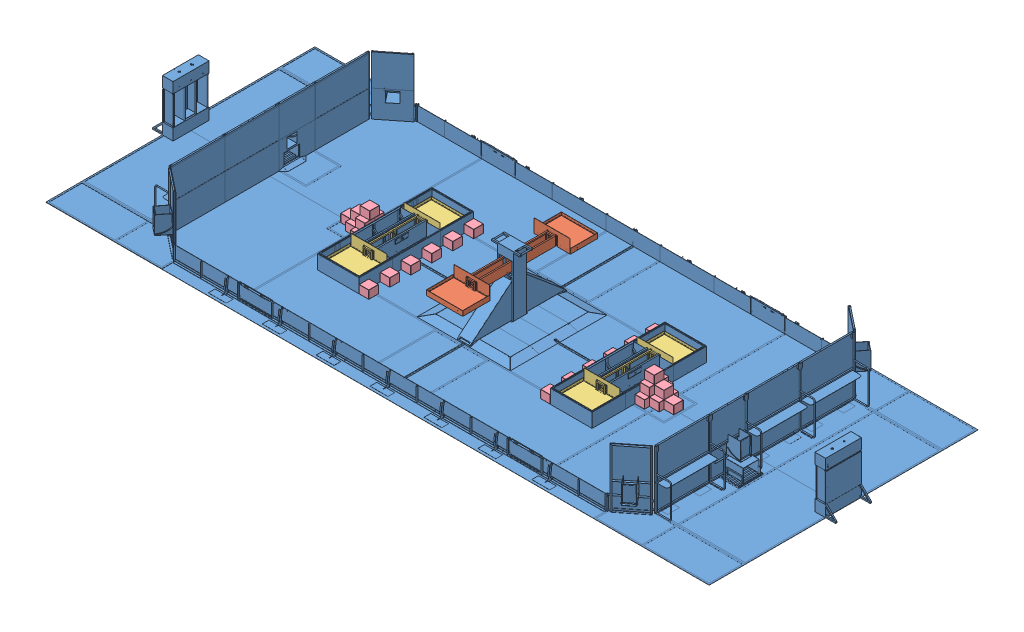
SolidWorks assembly FRC Field 2018a, configuration Arms Level. Lengths in mm.
Overall size (23234.65 2142.03 9144.04).
36 component instances, 4 part files, 15 mates.
Components (placement in the parent):
- FRC Fixed Field 2018-1: FRC Fixed Field 2018 [Default] at origin size (23234.65 2142.03 9144.04)
- Scale Arm-2: Scale Arm [Default] at (0 -0.1252 2.4571) x (1 0 0) z (0 0.001347 0.999999) size (1245.02 510 4602.7)
- Switch Arm-1: Switch Arm [Default] at (3962.4 0 -0.2032) size (1245.02 508 3684.03)
- Switch Arm-2: Switch Arm [Default] at (-3962.4 0 0) size (1245.02 508 3684.03)
- PowerUp Cube-1: PowerUp Cube [Default] at (4673.6 0 495.3) size (330.2 279.4 330.2)
- PowerUp Cube-2: PowerUp Cube [Default] at (4673.6 0 165.1) size (330.2 279.4 330.2)
- PowerUp Cube-3: PowerUp Cube [Default] at (4673.6 0 -165.1) size (330.2 279.4 330.2)
- PowerUp Cube-4: PowerUp Cube [Default] at (5003.8 0 330.2) size (330.2 279.4 330.2)
- PowerUp Cube-5: PowerUp Cube [Default] at (5003.8 0 0) size (330.2 279.4 330.2)
- PowerUp Cube-6: PowerUp Cube [Default] at (5334 0 165.1) size (330.2 279.4 330.2)
- PowerUp Cube-7: PowerUp Cube [Default] at (4673.6 279.4 330.2) size (330.2 279.4 330.2)
- PowerUp Cube-8: PowerUp Cube [Default] at (4673.6 279.4 0) size (330.2 279.4 330.2)
- PowerUp Cube-9: PowerUp Cube [Default] at (5003.8 279.4 165.1) size (330.2 279.4 330.2)
- PowerUp Cube-10: PowerUp Cube [Default] at (4673.6 558.8 165.1) size (330.2 279.4 330.2)
- PowerUp Cube-11: PowerUp Cube [Default] at (2921 0 -1619.25) size (330.2 279.4 330.2)
- PowerUp Cube-12: PowerUp Cube [Default] at (2921 0 -905.51) size (330.2 279.4 330.2)
- PowerUp Cube-13: PowerUp Cube [Default] at (2921 0 -191.77) size (330.2 279.4 330.2)
- PowerUp Cube-14: PowerUp Cube [Default] at (2921 0 521.97) size (330.2 279.4 330.2)
- PowerUp Cube-15: PowerUp Cube [Default] at (2921 0 1235.71) size (330.2 279.4 330.2)
- PowerUp Cube-16: PowerUp Cube [Default] at (2921 0 1949.45) size (330.2 279.4 330.2)
- PowerUp Cube-17: PowerUp Cube [Default] at (-4673.6 0 165.1) x (-1 0 0) z (0 0 -1) size (330.2 279.4 330.2)
- PowerUp Cube-18: PowerUp Cube [Default] at (-4673.6 0 -165.1) x (-1 0 0) z (0 0 -1) size (330.2 279.4 330.2)
- PowerUp Cube-19: PowerUp Cube [Default] at (-4673.6 0 -495.3) x (-1 0 0) z (0 0 -1) size (330.2 279.4 330.2)
- PowerUp Cube-20: PowerUp Cube [Default] at (-5003.8 0 0) x (-1 0 0) z (0 0 -1) size (330.2 279.4 330.2)
- PowerUp Cube-21: PowerUp Cube [Default] at (-5003.8 0 -330.2) x (-1 0 0) z (0 0 -1) size (330.2 279.4 330.2)
- PowerUp Cube-22: PowerUp Cube [Default] at (-5334 0 -165.1) x (-1 0 0) z (0 0 -1) size (330.2 279.4 330.2)
- PowerUp Cube-23: PowerUp Cube [Default] at (-4673.6 279.4 0) x (-1 0 0) z (0 0 -1) size (330.2 279.4 330.2)
- PowerUp Cube-24: PowerUp Cube [Default] at (-4673.6 279.4 -330.2) x (-1 0 0) z (0 0 -1) size (330.2 279.4 330.2)
- PowerUp Cube-25: PowerUp Cube [Default] at (-5003.8 279.4 -165.1) x (-1 0 0) z (0 0 -1) size (330.2 279.4 330.2)
- PowerUp Cube-26: PowerUp Cube [Default] at (-4673.6 558.8 -165.1) x (-1 0 0) z (0 0 -1) size (330.2 279.4 330.2)
- PowerUp Cube-27: PowerUp Cube [Default] at (-2921 0 -1949.45) x (-1 0 0) z (0 0 -1) size (330.2 279.4 330.2)
- PowerUp Cube-28: PowerUp Cube [Default] at (-2921 0 -1235.71) x (-1 0 0) z (0 0 -1) size (330.2 279.4 330.2)
- PowerUp Cube-29: PowerUp Cube [Default] at (-2921 0 -521.97) x (-1 0 0) z (0 0 -1) size (330.2 279.4 330.2)
- PowerUp Cube-30: PowerUp Cube [Default] at (-2921 0 191.77) x (-1 0 0) z (0 0 -1) size (330.2 279.4 330.2)
- PowerUp Cube-31: PowerUp Cube [Default] at (-2921 0 905.51) x (-1 0 0) z (0 0 -1) size (330.2 279.4 330.2)
- PowerUp Cube-32: PowerUp Cube [Default] at (-2921 0 1619.25) x (-1 0 0) z (0 0 -1) size (330.2 279.4 330.2)
Mates (geometry in assembly coordinates):
- Coincident1: coincident aligned: plane of FRC Fixed Field 2018-1 through (0 0 0) normal (0 1 0); plane of assembly through (0 0 0) normal (0 1 0)
- Coincident2: coincident aligned: plane of FRC Fixed Field 2018-1 through (0 0 0) normal (0 0 1); plane of assembly through (0 0 0) normal (0 0 1)
- Coincident3: coincident aligned: plane of FRC Fixed Field 2018-1 through (0 0 0) normal (1 0 0); plane of assembly through (0 0 0) normal (1 0 0)
- Distance1: distance = 19.05 mm anti-aligned: plane of Switch Arm-1 through (3810 460.502 -870.0516) normal (-1 0 0); plane of FRC Fixed Field 2018-1 through (3790.95 511.175 -838.2) normal (1 0 0)
- Concentric2: concentric aligned: cylinder of FRC Fixed Field 2018-1 through (3727.45 419.227 -0.1016) axis (1 0 0) radius 9.525; cylinder of Switch Arm-1 through (4140.2 419.227 -0.1016) axis (1 0 0) radius 19.05
- Distance2: distance = 19.05 mm anti-aligned: plane of FRC Fixed Field 2018-1 through (-4133.85 511.175 838.2) normal (1 0 0); plane of Switch Arm-2 through (-4114.8 460.502 -869.8484) normal (-1 0 0)
- Concentric3: concentric aligned: cylinder of FRC Fixed Field 2018-1 through (-3727.45 419.227 0.1016) axis (-1 0 0) radius 9.525; cylinder of Switch Arm-2 through (-4140.2 419.227 0.1016) axis (-1 0 0) radius 19.05
- Parallel1: parallel aligned: plane of FRC Fixed Field 2018-1 through (-11277.6 0 0) normal (0 1 0); plane of Switch Arm-2 through (-4092.575 482.727 -869.8484) normal (0 1 0)
- Parallel3: parallel aligned: plane of FRC Fixed Field 2018-1 through (-11277.6 0 0) normal (0 1 0); plane of Switch Arm-1 through (3832.225 482.727 -870.0516) normal (0 1 0)
- Distance4: distance = 381 mm: line of Switch Arm-2 through (-3365.5 381 -1832.1822) axis (-1 0 0); plane of FRC Fixed Field 2018-1 through (-11277.6 0 0) normal (0 1 0)
- Distance5: distance = 381 mm: line of Switch Arm-1 through (4559.3 381 -1832.3854) axis (-1 0 0); plane of FRC Fixed Field 2018-1 through (-11277.6 0 0) normal (0 1 0)
- Coincident4: coincident aligned: plane of Scale Arm-2; plane of assembly through (0 0 0) normal (1 0 0)
- Concentric4: concentric aligned: circle of FRC Fixed Field 2018-1; cylinder of Scale Arm-2 through (-158.75 1711.325 0) axis (1 0 0) radius 12.7
- Parallel4: parallel aligned: plane of FRC Fixed Field 2018-1 through (-11277.6 0 4572) normal (0 1 0); plane of Scale Arm-2 through (130.175 1774.825 1328.7375) normal (0 1 0)
- Distance6: distance = 1825.625 mm: line of Scale Arm-2 through (-596.9 1825.625 2286.6266) axis (1 0 0); plane of FRC Fixed Field 2018-1 through (-11277.6 0 4572) normal (0 1 0)
